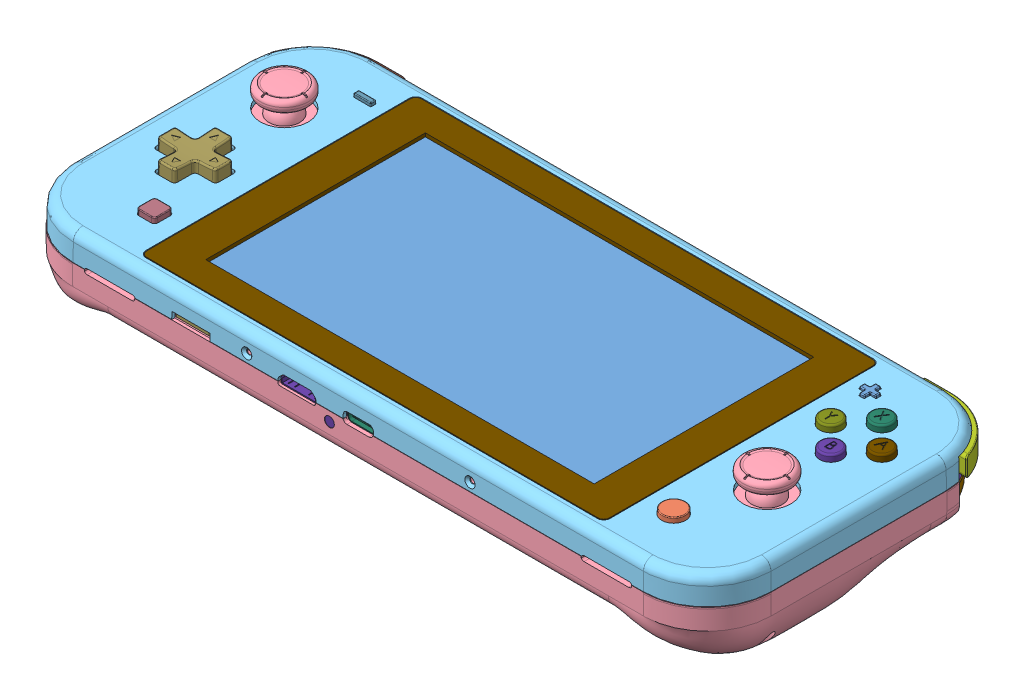
SolidWorks assembly Assembly Retro Lite CM5_1, configuration Default. Lengths in mm.
Overall size (229.59 38.19 107.71).
727 component instances, 202 part files, 109 mates.
Components (placement in the parent):
- Assembly Left PCB Controller-1: Assembly Left PCB Controller [Default] at (-1.1992 8.75 0) size (41.45 21.09 84.62)
  - MirrorSpeaker Assembly (2)-1: MirrorSpeaker Assembly (2) [Default] at (-72.5986 2.3241 29.1078) x (0 0 1) z (1 0 0) size (46.8 6.8 41.45)
    - MirrorSpeaker Duct (2)-1: MirrorSpeaker Duct (2) [Default] at (-0.5029 11.5241 -21.4164) size (46.4 3.6 41.45)
    - MirrorSpeaker Duct Lower (2)-1: MirrorSpeaker Duct Lower (2) [Default] at (-0.5029 8.3241 -21.4164) size (24.4 3.2 41.45)
  - Retrolite CM5 LCPCB v2 v1 (4)-1: Retrolite CM5 LCPCB v2 v1 (4) [Default] at (-63.231 -6 42.519) x (-1 0 0) z (0 -1 0) size (33.79 76.71 1.67)
    - Board (38)-1: Board (38) [Default] at origin size (33.79 76.71 1.67)
  - Switch Joystick Blank-2: Switch Joystick Blank [Default] at (-77.6 -0.75 -9.4) x (-1 0 0) z (0 0 1) size (24.9 13.52 30.9)
  - dualtact_BBStore v1-2: dualtact_BBStore v1 [Default] at (-2315.0854 1726.4 0.1557) x (-1 0 0) z (0 0 1) size (8.4 4.99 6.5)
  - 5034801700 v1-4: 5034801700 v1 [Default] at (-75.4873 -8.0211 10.6136) x (0 0 1) z (1 0 0) size (10.2 1.87 3.6)
  - 505110-0592 v1-2: 505110-0592 v1 [Default] at (-100.2545 -7.9954 -1.4465) x (1 0 0) z (0 0 -1) size (8 1.9 5.3)
  - Printed-Speaker-Duct-Lid-Mirrored v1-1: Printed-Speaker-Duct-Lid-Mirrored v1 [Default] at (-1072.2209 37.1812 -2157.2951) x (-1 0 0) z (0 0 1) size (19.6 1 43.54)
  - Single Silicone Cap-1: Single Silicone Cap [Default] at (-82.151 -6.3731 -29.942) size (8.6 3.9 8)
  - 436333033816 v1-2: 436333033816 v1 [Default] at (-91.1876 -6 -36.9451) x (-0.913545 0 0.406737) z (-0.406737 0 -0.913545) size (4.45 3.8 3.5)
  - Retro Lite CM5 (Latest)-1: Retro Lite CM5 (Latest) [Default] at origin size (6.6 3.1 6)
  - Retro Lite CM5 (Latest)-6-1: Retro Lite CM5 (Latest)-6 [Default] at origin size (6.6 3.1 6)
  - Retro Lite CM5 (Latest)-7-1: Retro Lite CM5 (Latest)-7 [Default] at origin size (6.6 3.1 6)
  - Retro Lite CM5 (Latest)-8-1: Retro Lite CM5 (Latest)-8 [Default] at origin size (6.6 3.1 6)
  - Retro Lite CM5 (Latest)-9-1: Retro Lite CM5 (Latest)-9 [Default] at origin size (6.6 3.1 6)
  - Retro Lite CM5 (Latest)-10-1: Retro Lite CM5 (Latest)-10 [Default] at origin size (6 3.1 6.6)
- Assembly Right PCB Controller-1: Assembly Right PCB Controller [Default] at (1.1992 8.75 0) size (41.45 21.27 84.19)
  - Speaker Assembly-1: Speaker Assembly [Default] at (72.5986 2.3241 29.1078) x (0 0 1) z (1 0 0) size (46.41 6.8 41.45)
    - Speaker Duct-1: Speaker Duct [Default] at (-0.5029 11.5241 21.4164) size (46.4 3.6 41.45)
    - Speaker Duct Lower-1: Speaker Duct Lower [Default] at (-0.5029 8.3241 21.4164) size (24.01 3.2 41.45)
  - Retrolite CM5 RCPCB v1 - RP2040 v2-1: Retrolite CM5 RCPCB v1 - RP2040 v2 [Default] at (55.135 -8.07 41.5) x (1 0 0) z (0 1 0) size (39.48 76.14 1.67)
    - Board (39)-1: Board (39) [Default] at origin size (39.48 76.14 1.67)
  - RESET (rev1) v1-1: RESET (rev1) v1 [Default] at (67.8813 -8 -22.9467) x (1 0 0) z (0 0 -1) size (3.2 2.5 4.6)
    - Frame-1: Frame [Default] at origin size (3.2 1.8 4.2)
    - Cover-1: Cover [Default] at (0 1.4 0) size (3 0.2 4.1)
    - Stem-1: Stem [Default] at (0 1.4 0) x (-1 0 0) z (0 0 -1) size (2.4 1.6 3.45)
    - Terminal-1: Terminal [Default] at (1.075 0.1 -2.0046) x (0 0 -1) z (0 1 0) size (1.2 0.55 0.5)
    - Terminal-2: Terminal [Default] at (-1.075 0.1 -2.0046) x (0 0 -1) z (0 1 0) size (1.2 0.55 0.5)
    - Terminal-3: Terminal [Default] at (1.075 0.1 2.0046) x (0 0 1) z (0 1 0) size (1.2 0.55 0.5)
    - Terminal-4: Terminal [Default] at (-1.075 0.1 2.0046) x (0 0 1) z (0 1 0) size (1.2 0.55 0.5)
  - RESET (rev1) v1-2: RESET (rev1) v1 [Default] at (67.8813 -8 -14.9467) x (1 0 0) z (0 0 -1) size (3.2 2.5 4.6)
    - Frame-1: Frame [Default] at origin size (3.2 1.8 4.2)
    - Cover-1: Cover [Default] at (0 1.4 0) size (3 0.2 4.1)
    - Stem-1: Stem [Default] at (0 1.4 0) x (-1 0 0) z (0 0 -1) size (2.4 1.6 3.45)
    - Terminal-1: Terminal [Default] at (1.075 0.1 -2.0046) x (0 0 -1) z (0 1 0) size (1.2 0.55 0.5)
    - Terminal-2: Terminal [Default] at (-1.075 0.1 -2.0046) x (0 0 -1) z (0 1 0) size (1.2 0.55 0.5)
    - Terminal-3: Terminal [Default] at (1.075 0.1 2.0046) x (0 0 1) z (0 1 0) size (1.2 0.55 0.5)
    - Terminal-4: Terminal [Default] at (-1.075 0.1 2.0046) x (0 0 1) z (0 1 0) size (1.2 0.55 0.5)
  - Switch Joystick Blank-1: Switch Joystick Blank [Default] at (77.6 -0.75 -0.6) x (1 0 0) z (0 0 -1) size (24.9 13.52 30.9)
  - dualtact_BBStore v1-1: dualtact_BBStore v1 [Default] at (-2141.3113 1726.42 0.1565) x (-1 0 0) z (0 0 1) size (8.4 4.99 6.5)
  - MPU-6050--3DModel-STEP-1 v1-1: MPU-6050--3DModel-STEP-1 v1 [Default] at (72.9128 -8.04 -5.7031) x (-1 0 0) z (0 0 1) size (4 0.95 4)
  - 5034801700 v1-3: 5034801700 v1 [Default] at (69.9408 -8.0211 10.3615) x (0 0 -1) z (-1 0 0) size (10.2 1.87 3.6)
  - 505110-0592 v1-1: 505110-0592 v1 [Default] at (100.3223 -7.9954 -6.8551) x (-1 0 0) z (0 0 1) size (8 1.9 5.3)
  - Printed-Speaker-Duct-Lid v1-1: Printed-Speaker-Duct-Lid v1 [Default] at (190.2814 -8 -197.965) x (-1 0 0) z (0 0 1) size (19.6 1 43.54)
  - Single Silicone Cap-2: Single Silicone Cap [Default] at (73.585 -6.3731 -29.8353) size (8.6 3.9 8)
  - RP2040_QFN_PACKAGE v1-1: RP2040_QFN_PACKAGE v1 [Default] at (84.645 -7.9955 -10.956) x (-1 0 0) z (0 -1 0) size (7.02 7.02 1)
  - 436333033816 v1-1: 436333033816 v1 [Default] at (91.1552 -6.4 -37.1789) x (-0.91706 0 -0.398749) z (0.398749 0 -0.91706) size (4.45 3.8 3.5)
  - Retro Lite CM5 (Latest)-11-1: Retro Lite CM5 (Latest)-11 [Default] at origin size (6.6 3.1 6)
  - Retro Lite CM5 (Latest)-12-1: Retro Lite CM5 (Latest)-12 [Default] at origin size (6.6 3.1 6)
  - Retro Lite CM5 (Latest)-13-1: Retro Lite CM5 (Latest)-13 [Default] at origin size (6.6 3.1 6)
  - Retro Lite CM5 (Latest)-14-1: Retro Lite CM5 (Latest)-14 [Default] at origin size (6.6 3.1 6)
  - Retro Lite CM5 (Latest)-15-1: Retro Lite CM5 (Latest)-15 [Default] at origin size (6 3.1 6.6)
  - Retro Lite CM5 (Latest)-16-1: Retro Lite CM5 (Latest)-16 [Default] at origin size (6.6 3.1 6)
  - Retro Lite CM5 (Latest)-17-1: Retro Lite CM5 (Latest)-17 [Default] at origin size (7.56 4.26 8.9)
- Assembly Center Components-1: Assembly Center Components [Default] at (0 9.4999 0) size (146.77 13.35 93.89)
  - Mini HDMI 685119136923-1: Mini HDMI 685119136923 [Default] at (-19.19 -7.55 40.38) x (0 0 1) z (0 -1 0) size (7.9 11.25 5.45)
    - Mini HDMI 685119136923(1)-1: Mini HDMI 685119136923(1) [Default] at origin size (7.9 11.25 5.45)
      - Housing-1: Housing [Default] at origin size (5.5 11.25 2.9)
      - Shielding-1: Shielding [Default] at (2.875 0 0.82) x (0 1 0) z (0 0 1) size (11.21 7.6 5.45)
      - Housing2-1: Housing2 [Default] at (-0.075 0 -0.65) x (0 -1 0) z (0 0 1) size (8.25 0.75 1.6)
      - Pin1-1: Pin1 [Default] at (2.1 -3.6 0.3) size (5.9 0.15 1.8)
      - Pin1-2: Pin1 [Default] at (2.1 -2.8 0.3) size (5.9 0.15 1.8)
      - Pin1-3: Pin1 [Default] at (2.1 -2.4 0.3) size (5.9 0.15 1.8)
      - Pin1-4: Pin1 [Default] at (2.1 -2 0.3) size (5.9 0.15 1.8)
      - Pin1-5: Pin1 [Default] at (2.1 -1.6 0.3) size (5.9 0.15 1.8)
      - Pin1-6: Pin1 [Default] at (2.1 -1.2 0.3) size (5.9 0.15 1.8)
      - Pin1-7: Pin1 [Default] at (2.1 -0.8 0.3) size (5.9 0.15 1.8)
      - Pin1-8: Pin1 [Default] at (2.1 -0.4 0.3) size (5.9 0.15 1.8)
      - Pin1-9: Pin1 [Default] at (2.1 0 0.3) size (5.9 0.15 1.8)
      - Pin1-10: Pin1 [Default] at (2.1 0.4 0.3) size (5.9 0.15 1.8)
      - Pin1-11: Pin1 [Default] at (2.1 0.8 0.3) size (5.9 0.15 1.8)
      - Pin1-12: Pin1 [Default] at (2.1 1.2 0.3) size (5.9 0.15 1.8)
      - Pin1-13: Pin1 [Default] at (2.1 1.6 0.3) size (5.9 0.15 1.8)
      - Pin1-14: Pin1 [Default] at (2.1 2 0.3) size (5.9 0.15 1.8)
      - Pin1-15: Pin1 [Default] at (2.1 2.4 0.3) size (5.9 0.15 1.8)
      - Pin1-16: Pin1 [Default] at (2.1 2.8 0.3) size (5.9 0.15 1.8)
      - Pin1-17: Pin1 [Default] at (2.1 3.2 0.3) size (5.9 0.15 1.8)
      - Pin1-18: Pin1 [Default] at (2.1 3.6 0.3) size (5.9 0.15 1.8)
      - Pin2-1: Pin2 [Default] at (1.7983 -3.2 0.3) size (5.3 0.15 1.8)
  - AX210 PCIe Card-1: AX210 PCIe Card [Default] at (0 25.3 -0.4) size (22 0.1 30)
    - Component473-1: Component473 [Default] at origin size (0.15 0.02 2.3)
    - Component424-1: Component424 [Default] at origin size (0.15 0.02 2.3)
    - Component429-1: Component429 [Default] at origin size (0.15 0.02 2.3)
    - Component423-1: Component423 [Default] at origin size (0.15 0.02 2.3)
    - Component430-1: Component430 [Default] at origin size (0.15 0.02 2.3)
    - Component431-1: Component431 [Default] at origin size (0.15 0.02 2.3)
    - Component426-1: Component426 [Default] at origin size (0.15 0.02 2.3)
    - Component422-1: Component422 [Default] at origin size (0.15 0.02 2.3)
    - Component425-1: Component425 [Default] at origin size (0.15 0.02 2.3)
    - Component428-1: Component428 [Default] at origin size (0.15 0.02 2.3)
    - Component446-1: Component446 [Default] at origin size (0.15 0.02 2.3)
    - Component448-1: Component448 [Default] at origin size (0.15 0.02 2.3)
    - Component449-1: Component449 [Default] at origin size (0.15 0.02 2.3)
    - Component443-1: Component443 [Default] at origin size (0.15 0.02 2.3)
    - Component442-1: Component442 [Default] at origin size (0.15 0.02 2.3)
    - Component447-1: Component447 [Default] at origin size (0.15 0.02 2.3)
    - Component451-1: Component451 [Default] at origin size (0.15 0.02 2.3)
    - Component450-1: Component450 [Default] at origin size (0.15 0.02 2.3)
    - Component445-1: Component445 [Default] at origin size (0.15 0.02 2.3)
    - Component472-1: Component472 [Default] at origin size (0.15 0.02 2.3)
    - Component408-1: Component408 [Default] at origin size (0.15 0.02 2.3)
    - Component409-1: Component409 [Default] at origin size (0.15 0.02 2.3)
    - Component410-1: Component410 [Default] at origin size (0.15 0.02 2.3)
    - Component405-1: Component405 [Default] at origin size (0.15 0.02 2.3)
    - Component411-1: Component411 [Default] at origin size (0.15 0.02 2.3)
    - Component403-1: Component403 [Default] at origin size (0.15 0.02 2.3)
    - Component406-1: Component406 [Default] at origin size (0.15 0.02 2.3)
    - Component404-1: Component404 [Default] at origin size (0.15 0.02 2.3)
    - Component407-1: Component407 [Default] at origin size (0.15 0.02 2.3)
    - Component400-1: Component400 [Default] at origin size (0.15 0.02 2.3)
    - Component401-1: Component401 [Default] at origin size (0.15 0.02 2.3)
    - Component433-1: Component433 [Default] at origin size (0.15 0.02 2.3)
    - Component437-1: Component437 [Default] at origin size (0.15 0.02 2.3)
    - Component438-1: Component438 [Default] at origin size (0.15 0.02 2.3)
    - Component436-1: Component436 [Default] at origin size (0.15 0.02 2.3)
    - Component434-1: Component434 [Default] at origin size (0.15 0.02 2.3)
    - Component439-1: Component439 [Default] at origin size (0.15 0.02 2.3)
    - Component440-1: Component440 [Default] at origin size (0.15 0.02 2.3)
    - Component435-1: Component435 [Default] at origin size (0.15 0.02 2.3)
    - Component458-1: Component458 [Default] at origin size (0.15 0.02 2.3)
    - Component460-1: Component460 [Default] at origin size (0.15 0.02 2.3)
    - Component456-1: Component456 [Default] at origin size (0.15 0.02 2.3)
    - Component457-1: Component457 [Default] at origin size (0.15 0.02 2.3)
    - Component461-1: Component461 [Default] at origin size (0.15 0.02 2.3)
    - Component452-1: Component452 [Default] at origin size (0.15 0.02 2.3)
    - Component453-1: Component453 [Default] at origin size (0.15 0.02 2.3)
    - Component455-1: Component455 [Default] at origin size (0.15 0.02 2.3)
    - Component465-1: Component465 [Default] at origin size (0.15 0.02 2.3)
    - Component468-1: Component468 [Default] at origin size (0.15 0.02 2.3)
    - Component467-1: Component467 [Default] at origin size (0.15 0.02 2.3)
    - Component464-1: Component464 [Default] at origin size (0.15 0.02 2.3)
    - Component469-1: Component469 [Default] at origin size (0.15 0.02 2.3)
    - Component470-1: Component470 [Default] at origin size (0.15 0.02 2.3)
    - Component471-1: Component471 [Default] at origin size (0.15 0.02 2.3)
    - Component462-1: Component462 [Default] at origin size (0.15 0.02 2.3)
    - Component463-1: Component463 [Default] at origin size (0.15 0.02 2.3)
    - Component466-1: Component466 [Default] at origin size (0.15 0.02 2.3)
    - Component413-1: Component413 [Default] at origin size (0.15 0.02 2.3)
    - Component417-1: Component417 [Default] at origin size (0.15 0.02 2.3)
    - Component414-1: Component414 [Default] at origin size (0.15 0.02 2.3)
    - Component415-1: Component415 [Default] at origin size (0.15 0.02 2.3)
    - Component421-1: Component421 [Default] at origin size (0.15 0.02 2.3)
    - Component418-1: Component418 [Default] at origin size (0.15 0.02 2.3)
    - Component419-1: Component419 [Default] at origin size (0.15 0.02 2.3)
    - Component420-1: Component420 [Default] at origin size (0.15 0.02 2.3)
    - Component412-1: Component412 [Default] at origin size (0.15 0.02 2.3)
    - AX210 PCIe Card-0-1: AX210 PCIe Card-0 [Default] at origin size (0.15 0.02 2.3)
    - AX210 PCIe Card-1-1: AX210 PCIe Card-1 [Default] at origin size (5.53 0.08 2.73)
    - AX210 PCIe Card-2-1: AX210 PCIe Card-2 [Default] at origin size (22 0.08 30)
  - 5.5_ Touch Display MIPI-1: 5.5_ Touch Display MIPI [Default] at origin size (145.01 5.25 86.09)
    - CTP-1: CTP [Default] at origin size (145.01 1.1 86.09)
    - 5.5_ Touch Display MIPI-3-1: 5.5_ Touch Display MIPI-3 [Default] at origin size (133.31 3.65 74.36)
    - 5.5_ Touch Display MIPI-4-1: 5.5_ Touch Display MIPI-4 [Default] at origin size (45 0.5 15.5)
    - 5.5_ Touch Display MIPI-5-1: 5.5_ Touch Display MIPI-5 [Default] at origin size (53.5 0.5 4.5)
  - RNQ0040A v1-1: RNQ0040A v1 [Default] at (1.8323 -6.1 22.7032) x (1 0 0) z (0 -1 0) size (6 4 0.8)
    - BODY-QFN-1: BODY-QFN [Default] at (0 0 0.025) x (1 0 0) z (0 -1 0) size (6 0.78 4)
    - FRAME-RNQ0040A-1: FRAME-RNQ0040A [Default] x (1 0 0) z (0 -1 0) size (6 0.2 4)
  - Radxa CM3-1: Radxa CM3 [Default] at (-34.1679 -8.7691 -17.6603) x (0 0 -1) z (0 -1 0) size (40.05 55.02 3.7)
    - Board_Geoms-1: Board_Geoms [Default] at origin size (40.05 55.02 1.2)
      - Board_outline-1: Board_outline [Default] at origin size (40.05 55.02 1.2)
    - EMP_Models-1: EMP_Models [Default] at origin size (39.5 54.73 3.7)
      - ANT2-1: ANT2 [Default] at (-11.75 25.8 0) size (4.01 3.43 1.3)
      - C1-1: C1 [Default] at (-3.8475 -1.7481 -1.2) x (-0.707107 -0.707107 0) z (0 0 -1) size (1.7 0.9 0.5)
      - C10-1: C10 [Default] at (3.3025 0.0519 -1.2) x (0.707107 0.707107 0) z (0 0 -1) size (1.1 0.6 0.35)
      - C10-2: C10 [Default] at (10.95 15.45 -1.2) x (0 1 0) z (0 0 -1) size (1.1 0.6 0.35)
      - C10-3: C10 [Default] at (3.8025 -0.3981 -1.2) x (-0.707107 -0.707107 0) z (0 0 -1) size (1.1 0.6 0.35)
      - C10-4: C10 [Default] at (-3.9975 -0.8481 -1.2) x (0.707107 0.707107 0) z (0 0 -1) size (1.1 0.6 0.35)
      - C1-2: C1 [Default] at (-14.1389 2.0823 0) x (0 1 0) z (0 0 1) size (1.7 0.9 0.5)
      - C10-5: C10 [Default] at (-4.6975 -21.9981 -1.2) x (0.707107 0.707107 0) z (0 0 -1) size (1.1 0.6 0.35)
      - C105-1: C105 [Default] at (13.9593 20.2111 -1.2) x (1 0 0) z (0 0 -1) size (2.5 1.3 0.6)
      - C105-2: C105 [Default] at (0.7006 -26.6671 0) size (2.5 1.3 0.6)
      - C105-3: C105 [Default] at (3.9693 -10.6117 -1.2) x (0 1 0) z (0 0 -1) size (2.5 1.3 0.6)
      - C10-6: C10 [Default] at (-3.0975 -8.9981 -1.2) x (0 1 0) z (0 0 -1) size (1.1 0.6 0.35)
      - C10-7: C10 [Default] at (-2.3475 -3.2981 -1.2) x (-0.707107 -0.707107 0) z (0 0 -1) size (1.1 0.6 0.35)
      - C1-3: C1 [Default] at (3.0025 0.7019 -1.2) x (0.707107 0.707107 0) z (0 0 -1) size (1.7 0.9 0.5)
      - C10-8: C10 [Default] at (-1.4475 -4.5481 -1.2) x (-0.707107 -0.707107 0) z (0 0 -1) size (1.1 0.6 0.35)
      - C10-9: C10 [Default] at (0.4525 -5.1481 -1.2) x (-0.707107 -0.707107 0) z (0 0 -1) size (1.1 0.6 0.35)
      - C10-10: C10 [Default] at (1.1525 -20.3481 -1.2) x (0 1 0) z (0 0 -1) size (1.1 0.6 0.35)
      - C10-11: C10 [Default] at (-2.0975 -16.8481 -1.2) x (0 1 0) z (0 0 -1) size (1.1 0.6 0.35)
      - C10-12: C10 [Default] at (-8.6975 -22.5481 -1.2) x (0.707107 -0.707107 0) z (0 0 -1) size (1.1 0.6 0.35)
      - C10-13: C10 [Default] at (-1.7475 -19.9981 -1.2) x (0.707107 -0.707107 0) z (0 0 -1) size (1.1 0.6 0.35)
      - C10-14: C10 [Default] at (2.6525 -20.0481 -1.2) x (1 0 0) z (0 0 -1) size (1.1 0.6 0.35)
      - C10-15: C10 [Default] at (6.7025 -17.4981 -1.2) x (0 1 0) z (0 0 -1) size (1.1 0.6 0.35)
      - C10-16: C10 [Default] at (-3.1475 -12.2481 0) x (0 -1 0) z (0 0 1) size (1.1 0.6 0.35)
      - C10-17: C10 [Default] at (-2.4475 -25.0481 -1.2) x (0.707107 -0.707107 0) z (0 0 -1) size (1.1 0.6 0.35)
      - C105-4: C105 [Default] at (0.9025 1.6519 -1.2) x (-0.707107 0.707107 0) z (0 0 -1) size (2.5 1.3 0.6)
      - C10-18: C10 [Default] at (-3.9475 -20.1981 -1.2) x (-0.707107 0.707107 0) z (0 0 -1) size (1.1 0.6 0.35)
      - C10-19: C10 [Default] at (6.3025 -22.0481 -1.2) x (0 -1 0) z (0 0 -1) size (1.1 0.6 0.35)
      - C10-20: C10 [Default] at (2.2025 -13.4481 -1.2) x (0 1 0) z (0 0 -1) size (1.1 0.6 0.35)
      - C10-21: C10 [Default] at (-3.4975 -13.6981 -1.2) x (0 1 0) z (0 0 -1) size (1.1 0.6 0.35)
      - C10-22: C10 [Default] at (-0.8475 -23.4481 -1.2) x (0.707107 -0.707107 0) z (0 0 -1) size (1.1 0.6 0.35)
      - C105-5: C105 [Default] at (3.682 -21.4585 -1.2) x (-1 0 0) z (0 0 -1) size (2.5 1.3 0.6)
      - C105-6: C105 [Default] at (-7.2334 -17.3788 -1.2) x (0 1 0) z (0 0 -1) size (2.5 1.3 0.6)
      - C105-7: C105 [Default] at (-10.5087 -5.7093 -1.2) x (-0.707107 -0.707107 0) z (0 0 -1) size (2.5 1.3 0.6)
      - C10-23: C10 [Default] at (8.2025 -12.0481 -1.2) x (0 1 0) z (0 0 -1) size (1.1 0.6 0.35)
      - C10-24: C10 [Default] at (-0.6475 -3.2981 -1.2) x (-0.707107 -0.707107 0) z (0 0 -1) size (1.1 0.6 0.35)
      - C105-8: C105 [Default] at (9 7.85 -1.2) x (1 0 0) z (0 0 -1) size (2.5 1.3 0.6)
      - C10-25: C10 [Default] at (1.1025 -3.3981 -1.2) x (0.707107 -0.707107 0) z (0 0 -1) size (1.1 0.6 0.35)
      - C10-26: C10 [Default] at (1.5525 -2.8981 -1.2) x (0.707107 -0.707107 0) z (0 0 -1) size (1.1 0.6 0.35)
      - C10-27: C10 [Default] at (5.7025 -24.2481 -1.2) x (-1 0 0) z (0 0 -1) size (1.1 0.6 0.35)
      - C10-28: C10 [Default] at (-9.6087 -6.0593 -1.2) x (-0.707107 -0.707107 0) z (0 0 -1) size (1.1 0.6 0.35)
      - C10-29: C10 [Default] at (5.3525 -16.2481 -1.2) x (0.707107 0.707107 0) z (0 0 -1) size (1.1 0.6 0.35)
      - C10-30: C10 [Default] at (4.1025 -19.8481 -1.2) x (0 -1 0) z (0 0 -1) size (1.1 0.6 0.35)
      - C10-31: C10 [Default] at (5.2525 -18.4981 -1.2) x (-1 0 0) z (0 0 -1) size (1.1 0.6 0.35)
      - C10-32: C10 [Default] at (-7.9475 -21.8981 -1.2) x (-0.707107 0.707107 0) z (0 0 -1) size (1.1 0.6 0.35)
      - C10-33: C10 [Default] at (-7.8975 -11.9481 -1.2) x (-0.707107 -0.707107 0) z (0 0 -1) size (1.1 0.6 0.35)
      - C10-34: C10 [Default] at (2.8025 -23.5481 -1.2) x (0 -1 0) z (0 0 -1) size (1.1 0.6 0.35)
      - C10-35: C10 [Default] at (-2.6475 1.2519 -1.2) x (0.707107 -0.707107 0) z (0 0 -1) size (1.1 0.6 0.35)
      - C10-36: C10 [Default] at (4.0025 -24.9981 -1.2) x (-1 0 0) z (0 0 -1) size (1.1 0.6 0.35)
      - C10-37: C10 [Default] at (-12.1475 -16.9481 -1.2) x (0 -1 0) z (0 0 -1) size (1.1 0.6 0.35)
      - C10-38: C10 [Default] at (4.2525 -14.4981 -1.2) x (1 0 0) z (0 0 -1) size (1.1 0.6 0.35)
      - C10-39: C10 [Default] at (8.2025 -19.6981 -1.2) x (0 1 0) z (0 0 -1) size (1.1 0.6 0.35)
      - C10-40: C10 [Default] at (3.8025 -17.7981 -1.2) x (1 0 0) z (0 0 -1) size (1.1 0.6 0.35)
      - C10-41: C10 [Default] at (-7.0975 -20.8481 -1.2) x (-0.707107 0.707107 0) z (0 0 -1) size (1.1 0.6 0.35)
      - C10-42: C10 [Default] at (-6.5975 -15.0481 -1.2) x (-0.707107 0.707107 0) z (0 0 -1) size (1.1 0.6 0.35)
      - C105-9: C105 [Default] at (11.9 -25.25 -1.2) x (1 0 0) z (0 0 -1) size (2.5 1.3 0.6)
      - C10-43: C10 [Default] at (-2.9975 -22.1481 -1.2) x (1 0 0) z (0 0 -1) size (1.1 0.6 0.35)
      - C10-44: C10 [Default] at (-17.9 -20.3 -1.2) x (1 0 0) z (0 0 -1) size (1.1 0.6 0.35)
      - C105-10: C105 [Default] at (-1.4475 2.3019 -1.2) x (0.707107 0.707107 0) z (0 0 -1) size (2.5 1.3 0.6)
      - C105-11: C105 [Default] at (1.5025 -25.9481 -1.2) x (1 0 0) z (0 0 -1) size (2.5 1.3 0.6)
      - C10-45: C10 [Default] at (3.4525 -15.6981 -1.2) x (1 0 0) z (0 0 -1) size (1.1 0.6 0.35)
      - C10-46: C10 [Default] at (-4.7975 -24.2981 -1.2) x (-0.707107 -0.707107 0) z (0 0 -1) size (1.1 0.6 0.35)
      - C10-47: C10 [Default] at (12.7525 -26.8981 -1.2) x (1 0 0) z (0 0 -1) size (1.1 0.6 0.35)
      - C105-12: C105 [Default] at (8.9525 -25.6481 -1.2) x (0 1 0) z (0 0 -1) size (2.5 1.3 0.6)
      - C1-4: C1 [Default] at (-15.75 -20.3 -1.2) x (-1 0 0) z (0 0 -1) size (1.7 0.9 0.5)
      - C105-13: C105 [Default] at (-4.3502 -26.0128 -1.2) x (-0.707107 -0.707107 0) z (0 0 -1) size (2.5 1.3 0.6)
      - C10-48: C10 [Default] at (2.5525 -18.8981 -1.2) x (1 0 0) z (0 0 -1) size (1.1 0.6 0.35)
      - C10-49: C10 [Default] at (1.7025 -23.5481 -1.2) x (0 1 0) z (0 0 -1) size (1.1 0.6 0.35)
      - C10-50: C10 [Default] at (-4.6475 -15.4981 -1.2) x (0 1 0) z (0 0 -1) size (1.1 0.6 0.35)
      - C105-14: C105 [Default] at (-2.8975 3.4519 -1.2) x (-0.707107 0.707107 0) z (0 0 -1) size (2.5 1.3 0.6)
      - C10-51: C10 [Default] at (-15.6 -16.6 -1.2) x (-1 0 0) z (0 0 -1) size (1.1 0.6 0.35)
      - C10-52: C10 [Default] at (11.5525 -22.4481 0) x (-1 0 0) z (0 0 1) size (1.1 0.6 0.35)
      - C10-53: C10 [Default] at (-17.25 -16.6 -1.2) x (1 0 0) z (0 0 -1) size (1.1 0.6 0.35)
      - C10-54: C10 [Default] at (-9.6071 3.2927 -1.2) x (0 1 0) z (0 0 -1) size (1.1 0.6 0.35)
      - C10-55: C10 [Default] at (-10.9034 6.1115 -1.2) x (0 1 0) z (0 0 -1) size (1.1 0.6 0.35)
      - C1-5: C1 [Default] at (-14.1734 12.7084 -1.2) x (0 -1 0) z (0 0 -1) size (1.7 0.9 0.5)
      - C1-6: C1 [Default] at (-5.1488 16.5367 0) x (0 1 0) z (0 0 1) size (1.7 0.9 0.5)
      - C10-56: C10 [Default] at (3.6525 -2.8981 -1.2) x (0.707107 0.707107 0) z (0 0 -1) size (1.1 0.6 0.35)
      - C1-7: C1 [Default] at (-7.1 20.8 0) size (1.7 0.9 0.5)
      - C10-57: C10 [Default] at (-8.4 20.75 0) x (-1 0 0) z (0 0 1) size (1.1 0.6 0.35)
      - C1-8: C1 [Default] at (6.8025 -3.5481 -1.2) x (-1 0 0) z (0 0 -1) size (1.7 0.9 0.5)
      - C10-58: C10 [Default] at (-5.1475 -1.2981 -1.2) x (-0.707107 0.707107 0) z (0 0 -1) size (1.1 0.6 0.35)
      - C10-59: C10 [Default] at (-14.45 -15.95 -1.2) x (1 0 0) z (0 0 -1) size (1.1 0.6 0.35)
      - C10-60: C10 [Default] at (13.1787 3.2726 -1.2) x (1 0 0) z (0 0 -1) size (1.1 0.6 0.35)
      - C105-15: C105 [Default] at (-14.4642 14.7415 -1.2) x (0 -1 0) z (0 0 -1) size (2.5 1.3 0.6)
      - C10-61: C10 [Default] at (-15.3485 19.4403 -1.2) x (0 1 0) z (0 0 -1) size (1.1 0.6 0.35)
      - C10-62: C10 [Default] at (-11.4987 22.5227 0) x (0 1 0) z (0 0 1) size (1.1 0.6 0.35)
      - C105-16: C105 [Default] at (-14.4738 19.5134 -1.2) x (0 1 0) z (0 0 -1) size (2.5 1.3 0.6)
      - C10-63: C10 [Default] at (-17.1616 18.5714 -1.2) x (1 0 0) z (0 0 -1) size (1.1 0.6 0.35)
      - C10-64: C10 [Default] at (-18.3116 18.5714 -1.2) x (-1 0 0) z (0 0 -1) size (1.1 0.6 0.35)
      - C10-65: C10 [Default] at (-19.0475 6.1019 0) x (-1 0 0) z (0 0 1) size (1.1 0.6 0.35)
      - C1-9: C1 [Default] at (5.4525 -4.1481 -1.2) x (0 1 0) z (0 0 -1) size (1.7 0.9 0.5)
      - C10-66: C10 [Default] at (-19.0475 6.7019 0) x (-1 0 0) z (0 0 1) size (1.1 0.6 0.35)
      - C10-67: C10 [Default] at (-17.8088 2.3575 0) x (-1 0 0) z (0 0 1) size (1.1 0.6 0.35)
      - C1-10: C1 [Default] at (-17.1397 6.6977 0) size (1.7 0.9 0.5)
      - C10-68: C10 [Default] at (-16.0385 6.7928 0) x (0 -1 0) z (0 0 1) size (1.1 0.6 0.35)
      - C10-69: C10 [Default] at (18.6 -11.05 0) x (0 1 0) z (0 0 1) size (1.1 0.6 0.35)
      - C10-70: C10 [Default] at (18.75 -15.6 0) size (1.1 0.6 0.35)
      - C10-71: C10 [Default] at (18.2 -16.1 -1.2) x (-1 0 0) z (0 0 -1) size (1.1 0.6 0.35)
      - C10-72: C10 [Default] at (18.75 -16.75 0) size (1.1 0.6 0.35)
      - C10-73: C10 [Default] at (18.75 -16.1 0) size (1.1 0.6 0.35)
      - C10-74: C10 [Default] at (-8.2975 -17.0981 -1.2) x (0 1 0) z (0 0 -1) size (1.1 0.6 0.35)
      - C10-75: C10 [Default] at (18.7502 -17.3853 0) size (1.1 0.6 0.35)
      - C1-11: C1 [Default] at (13.5025 -6.8481 0) size (1.7 0.9 0.5)
      - C1-12: C1 [Default] at (14.4525 -9.6481 0) size (1.7 0.9 0.5)
      - C10-76: C10 [Default] at (15.8525 -20.1981 0) x (0 -1 0) z (0 0 1) size (1.1 0.6 0.35)
      - C10-77: C10 [Default] at (15.8525 -20.1981 -1.2) x (0 -1 0) z (0 0 -1) size (1.1 0.6 0.35)
      - C1-13: C1 [Default] at (14.75 -11.85 -1.2) x (1 0 0) z (0 0 -1) size (1.7 0.9 0.5)
      - C1-14: C1 [Default] at (12.9525 -12.7981 -1.2) x (1 0 0) z (0 0 -1) size (1.7 0.9 0.5)
      - C10-78: C10 [Default] at (17.5 -13.4 -1.2) x (-1 0 0) z (0 0 -1) size (1.1 0.6 0.35)
      - C10-79: C10 [Default] at (12.8025 -13.5981 -1.2) x (1 0 0) z (0 0 -1) size (1.1 0.6 0.35)
      - C1-15: C1 [Default] at (18.8525 -20.0981 -1.2) x (-1 0 0) z (0 0 -1) size (1.7 0.9 0.5)
      - C1-16: C1 [Default] at (-3.0475 -2.3481 -1.2) x (-0.707107 -0.707107 0) z (0 0 -1) size (1.7 0.9 0.5)
      - C10-80: C10 [Default] at (0.4525 -18.5981 -1.2) x (-0.707107 -0.707107 0) z (0 0 -1) size (1.1 0.6 0.35)
      - C10-81: C10 [Default] at (18.9025 -20.8981 -1.2) x (-1 0 0) z (0 0 -1) size (1.1 0.6 0.35)
      - C10-82: C10 [Default] at (14.3025 -13.4481 -1.2) x (0 -1 0) z (0 0 -1) size (1.1 0.6 0.35)
      - C10-83: C10 [Default] at (12.8025 -14.2981 -1.2) x (1 0 0) z (0 0 -1) size (1.1 0.6 0.35)
      - C1-17: C1 [Default] at (17.0525 -20.0981 -1.2) x (1 0 0) z (0 0 -1) size (1.7 0.9 0.5)
      - C10-84: C10 [Default] at (16.5025 -20.1981 0) x (0 -1 0) z (0 0 1) size (1.1 0.6 0.35)
      - C10-85: C10 [Default] at (12.9025 -16.2481 -1.2) x (1 0 0) z (0 0 -1) size (1.1 0.6 0.35)
      - C10-86: C10 [Default] at (14.9912 -13.4244 -1.2) x (0 -1 0) z (0 0 -1) size (1.1 0.6 0.35)
      - C10-87: C10 [Default] at (17.5 -14.7 -1.2) x (-1 0 0) z (0 0 -1) size (1.1 0.6 0.35)
      - C10-88: C10 [Default] at (13.1025 -17.9981 -1.2) x (0 1 0) z (0 0 -1) size (1.1 0.6 0.35)
      - C10-89: C10 [Default] at (14.5525 -20.1981 0) x (0 -1 0) z (0 0 1) size (1.1 0.6 0.35)
      - C10-90: C10 [Default] at (0.0025 -12.9481 -1.2) x (0 1 0) z (0 0 -1) size (1.1 0.6 0.35)
      - C1-18: C1 [Default] at (-0.1475 -4.5981 -1.2) x (-0.707107 -0.707107 0) z (0 0 -1) size (1.7 0.9 0.5)
      - C10-91: C10 [Default] at (8.65 16.75 -1.2) x (-1 0 0) z (0 0 -1) size (1.1 0.6 0.35)
      - C10-92: C10 [Default] at (8.65 16.25 -1.2) x (-1 0 0) z (0 0 -1) size (1.1 0.6 0.35)
      - C105-17: C105 [Default] at (-17.9775 -6.6601 0) x (-0.707107 0.707107 0) z (0 0 1) size (2.5 1.3 0.6)
      - C105-18: C105 [Default] at (5.85 15.5 -1.2) x (0 1 0) z (0 0 -1) size (2.5 1.3 0.6)
      - C10-93: C10 [Default] at (3.7 14.75 -1.2) x (0 1 0) z (0 0 -1) size (1.1 0.6 0.35)
      - C10-94: C10 [Default] at (10.45 15.45 -1.2) x (0 1 0) z (0 0 -1) size (1.1 0.6 0.35)
      - C1-19: C1 [Default] at (10.6615 18.7103 -1.2) x (1 0 0) z (0 0 -1) size (1.7 0.9 0.5)
      - C10-95: C10 [Default] at (11.05 13.4 0) x (0 1 0) z (0 0 1) size (1.1 0.6 0.35)
      - C105-19: C105 [Default] at (9.65 12.3 -1.2) x (-1 0 0) z (0 0 -1) size (2.5 1.3 0.6)
      - C105-20: C105 [Default] at (0.1 0.75 -1.2) x (-0.707107 0.707107 0) z (0 0 -1) size (2.5 1.3 0.6)
      - C105-21: C105 [Default] at (-2.75 16.8 0) x (0 -1 0) z (0 0 1) size (2.5 1.3 0.6)
      - C105-22: C105 [Default] at (-4.1 16.8 0) x (0 -1 0) z (0 0 1) size (2.5 1.3 0.6)
      - C10-96: C10 [Default] at (8.5825 19.1459 -1.2) x (-1 0 0) z (0 0 -1) size (1.1 0.6 0.35)
      - C10-97: C10 [Default] at (8.55 19.8 -1.2) x (-1 0 0) z (0 0 -1) size (1.1 0.6 0.35)
      - C10-98: C10 [Default] at (8.6013 20.3134 -1.2) x (-1 0 0) z (0 0 -1) size (1.1 0.6 0.35)
      - C10-99: C10 [Default] at (3.2 14.75 -1.2) x (0 1 0) z (0 0 -1) size (1.1 0.6 0.35)
      - C105-23: C105 [Default] at (11.85 16.95 -1.2) x (1 0 0) z (0 0 -1) size (2.5 1.3 0.6)
      - C10-100: C10 [Default] at (3.75 13.1 0) x (0 -1 0) z (0 0 1) size (1.1 0.6 0.35)
      - C10-101: C10 [Default] at (3.95 11.35 0) x (-1 0 0) z (0 0 1) size (1.1 0.6 0.35)
      - C105-24: C105 [Default] at (9 9.05 -1.2) x (1 0 0) z (0 0 -1) size (2.5 1.3 0.6)
      - C105-25: C105 [Default] at (15.2 18.25 -1.2) x (0 -1 0) z (0 0 -1) size (2.5 1.3 0.6)
      - C10-102: C10 [Default] at (5.8 13.2 -1.2) x (0 -1 0) z (0 0 -1) size (1.1 0.6 0.35)
      - C10-103: C10 [Default] at (4.25 13.1 0) x (0 -1 0) z (0 0 1) size (1.1 0.6 0.35)
      - C105-26: C105 [Default] at (7.05 10.45 -1.2) x (0 1 0) z (0 0 -1) size (2.5 1.3 0.6)
      - C105-27: C105 [Default] at (-1.2753 -24.5477 -1.2) x (-0.707107 0.707107 0) z (0 0 -1) size (2.5 1.3 0.6)
      - C10-104: C10 [Default] at (2.9963 23.8177 0) x (0 1 0) z (0 0 1) size (1.1 0.6 0.35)
      - C105-28: C105 [Default] at (11.0433 21.7332 0) size (2.5 1.3 0.6)
      - C105-29: C105 [Default] at (2.5 20.95 -1.2) x (1 0 0) z (0 0 -1) size (2.5 1.3 0.6)
      - C10-105: C10 [Default] at (7.4413 23.0557 0) x (-1 0 0) z (0 0 1) size (1.1 0.6 0.35)
      - C10-106: C10 [Default] at (5.7 26.4 0) x (0 1 0) z (0 0 1) size (1.1 0.6 0.35)
      - C105-30: C105 [Default] at (2.5 19.75 -1.2) x (1 0 0) z (0 0 -1) size (2.5 1.3 0.6)
      - C105-31: C105 [Default] at (-4.1 20.65 0) x (0 -1 0) z (0 0 1) size (2.5 1.3 0.6)
      - C105-32: C105 [Default] at (-2.9 20.65 0) x (0 -1 0) z (0 0 1) size (2.5 1.3 0.6)
      - C10-107: C10 [Default] at (6.4683 25.0097 0) x (0 1 0) z (0 0 1) size (1.1 0.6 0.35)
      - C10-108: C10 [Default] at (9.4074 24.6986 0) x (0 1 0) z (0 0 1) size (1.1 0.6 0.35)
      - C10-109: C10 [Default] at (7.4413 23.9447 0) x (-1 0 0) z (0 0 1) size (1.1 0.6 0.35)
      - C10-110: C10 [Default] at (2.9963 24.9607 0) x (0 -1 0) z (0 0 1) size (1.1 0.6 0.35)
      - C105-33: C105 [Default] at (-5.35 24.95 0) size (2.5 1.3 0.6)
      - C10-111: C10 [Default] at (2.3613 23.8177 0) x (0 1 0) z (0 0 1) size (1.1 0.6 0.35)
      - C10-112: C10 [Default] at (1.1432 23.4631 0) size (1.1 0.6 0.35)
      - C10-113: C10 [Default] at (3.8853 24.9607 0) x (0 -1 0) z (0 0 1) size (1.1 0.6 0.35)
      - C10-114: C10 [Default] at (11.0479 19.812 -1.2) x (-1 0 0) z (0 0 -1) size (1.1 0.6 0.35)
      - C10-115: C10 [Default] at (0.0003 23.4631 0) x (-1 0 0) z (0 0 1) size (1.1 0.6 0.35)
      - C10-116: C10 [Default] at (4.5203 23.8177 0) x (0 -1 0) z (0 0 1) size (1.1 0.6 0.35)
      - C10-117: C10 [Default] at (1.6 16.7 -1.2) x (-1 0 0) z (0 0 -1) size (1.1 0.6 0.35)
      - C10-118: C10 [Default] at (5.2823 24.9607 0) x (0 -1 0) z (0 0 1) size (1.1 0.6 0.35)
      - C10-119: C10 [Default] at (3.8853 23.8177 0) x (0 1 0) z (0 0 1) size (1.1 0.6 0.35)
      - C10-120: C10 [Default] at (4.6473 24.9607 0) x (0 1 0) z (0 0 1) size (1.1 0.6 0.35)
      - C10-121: C10 [Default] at (-0.45 14.65 0) x (0 1 0) z (0 0 1) size (1.1 0.6 0.35)
      - C10-122: C10 [Default] at (-3.3387 23.8177 0) x (0 1 0) z (0 0 1) size (1.1 0.6 0.35)
      - C10-123: C10 [Default] at (-17.3087 -5.9093 0) x (-0.707107 0.707107 0) z (0 0 1) size (1.1 0.6 0.35)
      - C105-34: C105 [Default] at (7.9 17.65 -1.2) x (-1 0 0) z (0 0 -1) size (2.5 1.3 0.6)
      - C105-35: C105 [Default] at (17.8365 4.9199 0) x (0 -1 0) z (0 0 1) size (2.5 1.3 0.6)
      - C10-124: C10 [Default] at (17.9653 11.4831 0) size (1.1 0.6 0.35)
      - C105-36: C105 [Default] at (18.25 10.35 0) size (2.5 1.3 0.6)
      - C10-125: C10 [Default] at (-17.2504 -0.8345 0) x (-0.707107 -0.707107 0) z (0 0 1) size (1.1 0.6 0.35)
      - C105-37: C105 [Default] at (-12.05 -2.5 0) x (0.707107 -0.707107 0) z (0 0 1) size (2.5 1.3 0.6)
      - C105-38: C105 [Default] at (-14.7 -2.6 0) x (-0.707107 -0.707107 0) z (0 0 1) size (2.5 1.3 0.6)
      - C105-39: C105 [Default] at (-15.65 -1.6 0) x (-0.707107 -0.707107 0) z (0 0 1) size (2.5 1.3 0.6)
      - C10-126: C10 [Default] at (-17.6244 -3.2773 0) x (-0.707107 0.707107 0) z (0 0 1) size (1.1 0.6 0.35)
      - C10-127: C10 [Default] at (5 11.1 -1.2) x (0 -1 0) z (0 0 -1) size (1.1 0.6 0.35)
      - C10-128: C10 [Default] at (2.6 11.1 -1.2) x (0 -1 0) z (0 0 -1) size (1.1 0.6 0.35)
      - C10-129: C10 [Default] at (0.1 3.25 -1.2) x (-0.707107 -0.707107 0) z (0 0 -1) size (1.1 0.6 0.35)
      - C10-130: C10 [Default] at (3.4 11.1 -1.2) x (0 -1 0) z (0 0 -1) size (1.1 0.6 0.35)
      - C105-40: C105 [Default] at (-3.5 18.6 0) size (2.5 1.3 0.6)
      - C10-131: C10 [Default] at (14.25 -3.05 0) x (0 -1 0) z (0 0 1) size (1.1 0.6 0.35)
      - C105-41: C105 [Default] at (13.9025 -5.4981 0) size (2.5 1.3 0.6)
      - C10-132: C10 [Default] at (13.75 -4.65 0) size (1.1 0.6 0.35)
      - C105-42: C105 [Default] at (13.85 18.25 -1.2) x (0 -1 0) z (0 0 -1) size (2.5 1.3 0.6)
      - C10-133: C10 [Default] at (-5.2475 -23.8481 -1.2) x (-0.707107 -0.707107 0) z (0 0 -1) size (1.1 0.6 0.35)
      - C10-134: C10 [Default] at (-5.9475 -24.9981 -1.2) x (0.707107 -0.707107 0) z (0 0 -1) size (1.1 0.6 0.35)
      - C10-135: C10 [Default] at (5.3025 -8.0981 -1.2) x (1 0 0) z (0 0 -1) size (1.1 0.6 0.35)
      - C1-20: C1 [Default] at (0.5525 -2.4481 -1.2) x (0.707107 0.707107 0) z (0 0 -1) size (1.7 0.9 0.5)
      - C1-21: C1 [Default] at (-1.1651 -2.1207 -1.2) x (-0.707107 0.707107 0) z (0 0 -1) size (1.7 0.9 0.5)
      - C10-136: C10 [Default] at (0.1 14.65 0) x (0 1 0) z (0 0 1) size (1.1 0.6 0.35)
      - C105-43: C105 [Default] at (-3.5 0.5 -1.2) x (-0.707107 0.707107 0) z (0 0 -1) size (2.5 1.3 0.6)
      - C10-137: C10 [Default] at (-4.35 11.05 0) size (1.1 0.6 0.35)
      - C10-138: C10 [Default] at (-5.5038 11.0162 0) x (-1 0 0) z (0 0 1) size (1.1 0.6 0.35)
      - C10-139: C10 [Default] at (0.7025 5.2019 -1.2) x (0.707107 0.707107 0) z (0 0 -1) size (1.1 0.6 0.35)
      - C10-140: C10 [Default] at (-1.35 4.5 -1.2) x (-0.707107 -0.707107 0) z (0 0 -1) size (1.1 0.6 0.35)
      - C10-141: C10 [Default] at (-0.75 5.45 -1.2) x (0.707107 0.707107 0) z (0 0 -1) size (1.1 0.6 0.35)
      - C10-142: C10 [Default] at (-2.6 7.15 -1.2) x (-1 0 0) z (0 0 -1) size (1.1 0.6 0.35)
      - C10-143: C10 [Default] at (-1.7475 5.9519 -1.2) x (0.707107 -0.707107 0) z (0 0 -1) size (1.1 0.6 0.35)
      - C10-144: C10 [Default] at (8.25 14.15 -1.2) x (-1 0 0) z (0 0 -1) size (1.1 0.6 0.35)
      - C10-145: C10 [Default] at (-1.9975 4.1019 -1.2) x (0.707107 -0.707107 0) z (0 0 -1) size (1.1 0.6 0.35)
